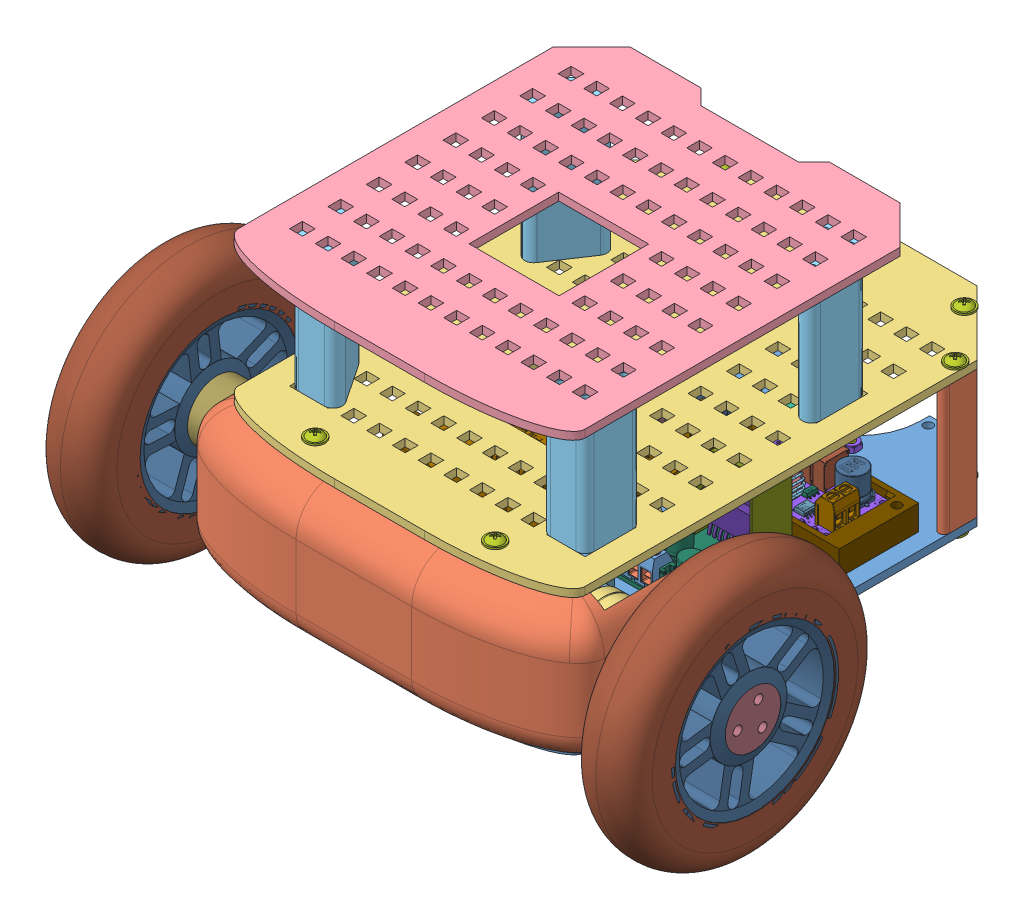
SolidWorks assembly main_assembly_generic, configuration Default. Lengths in mm.
Overall size (232.39 154.6 231.75).
188 component instances, 46 part files, 130 mates.
Components (placement in the parent):
- base_generic-1: base_generic [Predeterminado] at origin size (135.31 3.5 190.25)
- front_noah-1: front_noah [Predeterminado] at (0 3 75) size (155.37 50.11 66.16)
- JA25-371-12V-1: JA25-371-12V [Predeterminado] at (32.9354 21.1621 81.9623) x (0 0 -1) z (1 0 0) size (25 25 76.39)
  - Gearbox-1: Gearbox [Predeterminado] at (16.9623 5.2379 20.5646) size (25 25 21)
  - hub-1: hub [Predeterminado] at (16.9623 5.2379 39.5646) x (0.985611 -0.169031 0) z (0 0 1) size (6.95 6.95 4.5)
  - Motor-1: Motor [Predeterminado] at (16.9623 5.2379 -9.9354) size (24.2 24.2 30.5)
  - Axis-1: Axis [Predeterminado] at (16.9623 5.2379 39.5646) x (0.853161 0.521648 0) z (0 0 1) size (4 4 14)
  - PCB-1: PCB [Predeterminado] at (16.9623 5.2379 -11.4354) x (-1 0 0) z (0 0 -1) size (23 23 4.73)
  - Magnet-1: Magnet [Predeterminado] at (16.9623 5.2379 -17.3254) x (-0.17817 -0.984 0) z (0 0 -1) size (14.2 14.2 15.5)
- JA25-371-12V-2: JA25-371-12V [Predeterminado] at (-32.9354 21.1621 48.0377) x (0 0 1) z (-1 0 0) size (25 25 76.39)
  - Gearbox-1: Gearbox [Predeterminado] at (16.9623 5.2379 20.5646) size (25 25 21)
  - hub-1: hub [Predeterminado] at (16.9623 5.2379 39.5646) x (0.985611 -0.169031 0) z (0 0 1) size (6.95 6.95 4.5)
  - Motor-1: Motor [Predeterminado] at (16.9623 5.2379 -9.9354) size (24.2 24.2 30.5)
  - Axis-1: Axis [Predeterminado] at (16.9623 5.2379 39.5646) x (0.853161 0.521648 0) z (0 0 1) size (4 4 14)
  - PCB-1: PCB [Predeterminado] at (16.9623 5.2379 -11.4354) x (-1 0 0) z (0 0 -1) size (23 23 4.73)
  - Magnet-1: Magnet [Predeterminado] at (16.9623 5.2379 -17.3254) x (-0.17817 -0.984 0) z (0 0 -1) size (14.2 14.2 15.5)
- Arduino Uno-1: Arduino Uno [Default] at (-32.9854 13 -7.3988) x (0 0 -1) z (0 1 0) size (53 76.4 13)
- TuxsWheel100mm-1: TuxsWheel100mm [Default] at (-181.0669 -0.4628 121.5667) x (0 -0.425374 -0.905018) z (1 0 0) size (114.18 114.18 36.69)
  - B02-1: B02 [Default] at (39.7671 48.3733 64.9228) size (90.04 90.04 24)
  - B021-1: B021 [Default] at (39.7671 48.3733 64.9228) x (0.988174 0.153337 0) z (0 0 1) size (100.02 100.02 24.11)
  - Adapter1-1: Adapter1 [Default] at (39.7671 48.3733 72.3069) x (0 -1 0) z (0 0 1) size (23 23 29.26)
  - Adapter2-1: Adapter2 [Default] at (39.7671 48.3733 65.8069) x (0 -1 0) z (0 0 1) size (21.7 21.7 6.5)
  - countersunk flat head cross recess screw_din-6: countersunk flat head cross recess screw_din [DIN EN ISO 7046-1 - M3 x 10 - Z - 10C] at (51.0178 48.3733 97.0669) x (-1 0 0) z (0 -0.928088 -0.37236) size (10 5.5 5.5) (hidden)
  - countersunk flat head cross recess screw_din-7: countersunk flat head cross recess screw_din [DIN EN ISO 7046-1 - M3 x 10 - Z - 10C] at (28.4595 48.3733 97.0669) x (1 0 0) z (0 0.306192 0.95197) size (10 5.5 5.5) (hidden)
  - countersunk flat head cross recess screw_din-8: countersunk flat head cross recess screw_din [DIN EN ISO 7046-1 - M3 x 10 - Z - 10C] at (36.7671 53.5694 65.4069) x (0 0 1) z (-0.331366 0.943502 0) size (10 5.5 5.5) (hidden)
  - countersunk flat head cross recess screw_din-9: countersunk flat head cross recess screw_din [DIN EN ISO 7046-1 - M3 x 10 - Z - 10C] at (36.7671 43.1771 65.4069) x (0 0 1) z (-0.394756 0.918786 0) size (10 5.5 5.5) (hidden)
  - countersunk flat head cross recess screw_din-10: countersunk flat head cross recess screw_din [DIN EN ISO 7046-1 - M3 x 10 - Z - 10C] at (45.7671 48.3733 65.4069) x (0 0 1) z (0.637808 -0.770196 0) size (10 5.5 5.5) (hidden)
  - hex thin nut gradeb_din-1: hex thin nut gradeb_din [Hexagon Nut ISO 4036 - M3 - C] at (33.3451 48.3733 97.0669) x (0 -1 0) z (-1 0 0) size (5.5 6.35 1.8) (hidden)
  - hex thin nut gradeb_din-2: hex thin nut gradeb_din [Hexagon Nut ISO 4036 - M3 - C] at (44.1892 48.3733 97.0669) x (0 -1 0) z (-1 0 0) size (5.5 6.35 1.8) (hidden)
- TuxsWheel100mm-2: TuxsWheel100mm [Default] at (181.0669 87.718 52.2919) x (0 -0.778594 -0.627529) z (-1 0 0) size (114.18 114.18 36.69)
  - B02-1: B02 [Default] at (39.7671 48.3733 64.9228) size (90.04 90.04 24)
  - B021-1: B021 [Default] at (39.7671 48.3733 64.9228) x (0.988174 0.153337 0) z (0 0 1) size (100.02 100.02 24.11)
  - Adapter1-1: Adapter1 [Default] at (39.7671 48.3733 72.3069) x (0 -1 0) z (0 0 1) size (23 23 29.26)
  - Adapter2-1: Adapter2 [Default] at (39.7671 48.3733 65.8069) x (0 -1 0) z (0 0 1) size (21.7 21.7 6.5)
  - countersunk flat head cross recess screw_din-6: countersunk flat head cross recess screw_din [DIN EN ISO 7046-1 - M3 x 10 - Z - 10C] at (51.0178 48.3733 97.0669) x (-1 0 0) z (0 -0.928088 -0.37236) size (10 5.5 5.5) (hidden)
  - countersunk flat head cross recess screw_din-7: countersunk flat head cross recess screw_din [DIN EN ISO 7046-1 - M3 x 10 - Z - 10C] at (28.4595 48.3733 97.0669) x (1 0 0) z (0 0.306192 0.95197) size (10 5.5 5.5) (hidden)
  - countersunk flat head cross recess screw_din-8: countersunk flat head cross recess screw_din [DIN EN ISO 7046-1 - M3 x 10 - Z - 10C] at (36.7671 53.5694 65.4069) x (0 0 1) z (-0.331366 0.943502 0) size (10 5.5 5.5) (hidden)
  - countersunk flat head cross recess screw_din-9: countersunk flat head cross recess screw_din [DIN EN ISO 7046-1 - M3 x 10 - Z - 10C] at (36.7671 43.1771 65.4069) x (0 0 1) z (-0.394756 0.918786 0) size (10 5.5 5.5) (hidden)
  - countersunk flat head cross recess screw_din-10: countersunk flat head cross recess screw_din [DIN EN ISO 7046-1 - M3 x 10 - Z - 10C] at (45.7671 48.3733 65.4069) x (0 0 1) z (0.637808 -0.770196 0) size (10 5.5 5.5) (hidden)
  - hex thin nut gradeb_din-1: hex thin nut gradeb_din [Hexagon Nut ISO 4036 - M3 - C] at (33.3451 48.3733 97.0669) x (0 -1 0) z (-1 0 0) size (5.5 6.35 1.8) (hidden)
  - hex thin nut gradeb_din-2: hex thin nut gradeb_din [Hexagon Nut ISO 4036 - M3 - C] at (44.1892 48.3733 97.0669) x (0 -1 0) z (-1 0 0) size (5.5 6.35 1.8) (hidden)
- Spacer10mm-1: Spacer10mm [Varsayılan] at (-45 13 33) x (-0.837169 0 -0.546944) z (-0.546944 0 0.837169) size (5.71 16.2 5)
- Spacer10mm-2: Spacer10mm [Varsayılan] at (-45 13 -15.6) x (-0.837169 0 -0.546944) z (-0.546944 0 0.837169) size (5.71 16.2 5)
- Spacer10mm-3: Spacer10mm [Varsayılan] at (5.9048 13 -0.3747) x (-0.837169 0 -0.546944) z (-0.546944 0 0.837169) size (5.71 16.2 5)
- Spacer10mm-4: Spacer10mm [Varsayılan] at (5.9037 13 26.6253) x (-0.837169 0 -0.546944) z (-0.546944 0 0.837169) size (5.71 16.2 5)
- Montaj - L298 DC Motor Drive-1: Montaj - L298 DC Motor Drive [Varsayılan] at (35.2269 11.4274 -35.05) size (43.5 27 43.55)
  - L298 Board-1: L298 Board [Varsayılan] at (5.3531 1.5726 43.5) size (43.5 12.01 43.5)
  - Cooler Blok-1: Cooler Blok [Varsayılan] at (5.3531 27.5726 29.4518) x (-1 0 0) z (0 0 1) size (23 27 15.5)
  - L298N Regulator-1: L298N Regulator [Varsayılan] at (5.3531 16.3226 30.2018) size (21 23.01 4.5)
  - Vida M3x4.5-1: Vida M3x4.5 [Varsayılan] at (5.3531 22.0726 31.7018) size (5 5 6.5)
  - Clamp Body-1: Clamp Body [Varsayılan] at (-1.8969 8.5726 60.75) x (-1 0 0) z (0 0 -1) size (15 10.5 8)
  - Metal Clamp Part-1: Metal Clamp Part [Varsayılan] at (3.1031 6.5726 61.3938) size (4 11.02 6)
  - Metal Clamp Part-2: Metal Clamp Part [Varsayılan] at (-1.8969 6.5726 61.3938) size (4 11.02 6)
  - Metal Clamp Part-3: Metal Clamp Part [Varsayılan] at (-6.8969 6.5726 61.3938) size (4 11.02 6)
  - Clamp Body 2x-1: Clamp Body 2x [Varsayılan] at (-12.3969 8.5726 50.25) x (0 0 -1) z (1 0 0) size (10 10.5 8)
  - Metal Clamp Part-4: Metal Clamp Part [Varsayılan] at (-13.0407 6.5726 47.75) x (0 0 1) z (-1 0 0) size (4 11.02 6)
  - Metal Clamp Part-5: Metal Clamp Part [Varsayılan] at (-13.0407 6.5726 52.75) x (0 0 1) z (-1 0 0) size (4 11.02 6)
  - Clamp Body 2x-2: Clamp Body 2x [Varsayılan] at (23.1031 8.5726 50.25) x (0 0 1) z (-1 0 0) size (10 10.5 8)
  - Metal Clamp Part-6: Metal Clamp Part [Varsayılan] at (23.7469 6.5726 52.75) x (0 0 -1) z (1 0 0) size (4 11.02 6)
  - Metal Clamp Part-7: Metal Clamp Part [Varsayılan] at (23.7469 6.5726 47.75) x (0 0 -1) z (1 0 0) size (4 11.02 6)
- Spacer10mm-5: Spacer10mm [Varsayılan] at (20.83 13 28.2) x (-0.837169 0 -0.546944) z (-0.546944 0 0.837169) size (5.71 16.2 5)
- Spacer10mm-6: Spacer10mm [Varsayılan] at (20.83 13 -11.3) x (-0.837169 0 -0.546944) z (-0.546944 0 0.837169) size (5.71 16.2 5)
- Spacer10mm-7: Spacer10mm [Varsayılan] at (60.33 13 -11.3) x (-0.837169 0 -0.546944) z (-0.546944 0 0.837169) size (5.71 16.2 5)
- Spacer10mm-8: Spacer10mm [Varsayılan] at (60.33 13 28.2) x (-0.837169 0 -0.546944) z (-0.546944 0 0.837169) size (5.71 16.2 5)
- XL4015-1: XL4015 [Default] at (2.5 8.7 -25.3) x (1 0 0) z (0 1 0) size (51 26 18.44)
  - XL4015 StepDown DC-DC 5A (CC-CV) v1.step-1: XL4015 StepDown DC-DC 5A (CC-CV) v1.step [Default] at origin size (51 26 18.44)
    - Coil v9.step-1: Coil v9.step [Default] at (0 0 9) x (0 0 -1) z (0 -1 0) size (17.32 14.29 7.7)
      - Toro.step-1: Toro.step [Default] at (0.4 28 -5) size (13 12 6)
      - Spira.step-1: Spira.step [Default] at (0.4 28 -5) x (0.965926 0.258819 0) z (0 0 1) size (4.37 2.38 7.7)
      - Spira.step-2: Spira.step [Default] at (0.4 28 -5) x (0.866025 0.5 0) z (0 0 1) size (4.37 2.38 7.7)
      - Spira.step-3: Spira.step [Default] at (0.4 28 -5) x (0.707107 0.707107 0) z (0 0 1) size (4.37 2.38 7.7)
      - Spira.step-4: Spira.step [Default] at (0.4 28 -5) x (0.5 0.866025 0) z (0 0 1) size (4.37 2.38 7.7)
      - Spira.step-5: Spira.step [Default] at (0.4 28 -5) x (0.258819 0.965926 0) z (0 0 1) size (4.37 2.38 7.7)
      - Spira.step-6: Spira.step [Default] at (0.4 28 -5) x (0 1 0) z (0 0 1) size (4.37 2.38 7.7)
      - Spira.step-7: Spira.step [Default] at (0.4 28 -5) x (-0.258819 0.965926 0) z (0 0 1) size (4.37 2.38 7.7)
      - Spira.step-8: Spira.step [Default] at (0.4 28 -5) x (-0.5 0.866025 0) z (0 0 1) size (4.37 2.38 7.7)
      - Spira.step-9: Spira.step [Default] at (0.4 28 -5) x (-0.707107 0.707107 0) z (0 0 1) size (4.37 2.38 7.7)
      - Spira.step-10: Spira.step [Default] at (0.4 28 -5) x (-0.866025 0.5 0) z (0 0 1) size (4.37 2.38 7.7)
      - Spira.step-11: Spira.step [Default] at (0.4 28 -5) x (-0.965926 0.258819 0) z (0 0 1) size (4.37 2.38 7.7)
      - Spira.step-12: Spira.step [Default] at (0.4 28 -5) x (-1 0 0) z (0 0 1) size (4.37 2.38 7.7)
      - Spira.step-13: Spira.step [Default] at (0.4 28 -5) x (-0.965926 -0.258819 0) z (0 0 1) size (4.37 2.38 7.7)
      - Spira.step-14: Spira.step [Default] at (0.4 28 -5) x (-0.866025 -0.5 0) z (0 0 1) size (4.37 2.38 7.7)
      - Spira.step-15: Spira.step [Default] at (0.4 28 -5) x (-0.707107 -0.707107 0) z (0 0 1) size (4.37 2.38 7.7)
      - Spira.step-16: Spira.step [Default] at (0.4 28 -5) x (-0.5 -0.866025 0) z (0 0 1) size (4.37 2.38 7.7)
      - Spira.step-17: Spira.step [Default] at (0.4 28 -5) x (-0.258819 -0.965926 0) z (0 0 1) size (4.37 2.38 7.7)
      - Spira.step-18: Spira.step [Default] at (0.4 28 -5) x (0 -1 0) z (0 0 1) size (4.37 2.38 7.7)
      - Spira.step-19: Spira.step [Default] at (0.4 28 -5) x (0.258819 -0.965926 0) z (0 0 1) size (4.37 2.38 7.7)
      - Spira.step-20: Spira.step [Default] at (0.4 28 -5) x (0.5 -0.866025 0) z (0 0 1) size (4.37 2.38 7.7)
      - Spira.step-21: Spira.step [Default] at (0.4 28 -5) x (0.707107 -0.707107 0) z (0 0 1) size (4.37 2.38 7.7)
      - Spira.step-22: Spira.step [Default] at (0.4 28 -5) x (0.866025 -0.5 0) z (0 0 1) size (4.37 2.38 7.7)
      - SpiraCodA.step-1: SpiraCodA.step [Default] at (0.4015 27.9945 -5) x (1 0.000874 0) z (0 0 1) size (7.52 2.39 7.7)
      - SpiraCpdB.step-1: SpiraCpdB.step [Default] at (0.399 27.9963 -5) x (0.966079 -0.258245 0) z (0 0 1) size (7.28 3.27 7.7)
    - Basetta.step-1: Basetta.step [Default] at origin size (51 26 1.7)
    - DG301-5.0-02 v1.step-1: DG301-5.0-02 v1.step [Default] at (4 19.4 1.6) x (0 -1 0) z (0 0 1) size (10.6 7.6 14.3)
    - DG301-5.0-02 v1.step-2: DG301-5.0-02 v1.step [Default] at (47 6.6 1.6) x (0 1 0) z (0 0 1) size (10.6 7.6 14.3)
    - CAPACITOR 10x10 SMD v1.step-1: CAPACITOR 10x10 SMD v1.step [Default] at (9.325 5.925 1.6) x (1 0 0) z (0 -1 0) size (10.25 10.61 11.85)
    - CAPACITOR 10x10 SMD v1.step-2: CAPACITOR 10x10 SMD v1.step [Default] at (41.475 19.975 1.6) x (0 -1 0) z (-1 0 0) size (10.25 10.61 11.85)
    - Trimpot 3296W v1.step-1: Trimpot 3296W v1.step [Default] at (26.715 20.735 1.6) x (0 -1 0) z (0 0 1) size (9.56 4.83 14.15)
    - Trimpot 3296W v1.step-2: Trimpot 3296W v1.step [Default] at (32.265 20.735 1.6) x (0 -1 0) z (0 0 1) size (9.56 4.83 14.15)
    - DO-214AB v1.step-1: DO-214AB v1.step [Default] at (18.1 1.725 1.6) x (0 1 0) z (0 0 1) size (8.15 6.25 2.66)
    - XL4015 TO263-5-1 v1.step-1: XL4015 TO263-5-1 v1.step [Default] at (18.4666 17.0892 1.5654) x (0 -1 0) z (-0.006883 0 0.999976) size (9.82 14.6 4.22)
    - LM358 SOIC08 v1.step-1: LM358 SOIC08 v1.step [Default] at (37 6 1.55) x (0 -1 0) z (0 0 1) size (5 6.17 2.02)
    - UPC78L08T-E1-AZ.step-1: UPC78L08T-E1-AZ.step [Default] at (31.81 12.82 1.6) x (0 1 0) z (0 0 1) size (4.36 4 1.51)
    - SC-59A v1.step-1: SC-59A v1.step [Default] at (36.8 13.75 1.6) x (0 -1 0) z (0 0 1) size (3.1 3 1.45)
    - LED v1.step-1: LED v1.step [Default] at (44.84 1.625 1.62) x (0 -1 0) z (-1 0 0) size (1.27 0.67 2.02)
    - LED v1.step-2: LED v1.step [Default] at (39.84 1.625 1.62) x (0 -1 0) z (-1 0 0) size (1.27 0.67 2.02)
    - LED v1.step-3: LED v1.step [Default] at (20.16 23.875 1.62) x (0 -1 0) z (-1 0 0) size (1.27 0.67 2.02)
- XL4015-2: XL4015 [Default] at (-2.5 8.7 -51.3) x (-1 0 0) z (0 1 0) size (51 26 18.44)
  - XL4015 StepDown DC-DC 5A (CC-CV) v1.step-1: XL4015 StepDown DC-DC 5A (CC-CV) v1.step [Default] at origin size (51 26 18.44)
    - Coil v9.step-1: Coil v9.step [Default] at (0 0 9) x (0 0 -1) z (0 -1 0) size (17.32 14.29 7.7)
      - Toro.step-1: Toro.step [Default] at (0.4 28 -5) size (13 12 6)
      - Spira.step-1: Spira.step [Default] at (0.4 28 -5) x (0.965926 0.258819 0) z (0 0 1) size (4.37 2.38 7.7)
      - Spira.step-2: Spira.step [Default] at (0.4 28 -5) x (0.866025 0.5 0) z (0 0 1) size (4.37 2.38 7.7)
      - Spira.step-3: Spira.step [Default] at (0.4 28 -5) x (0.707107 0.707107 0) z (0 0 1) size (4.37 2.38 7.7)
      - Spira.step-4: Spira.step [Default] at (0.4 28 -5) x (0.5 0.866025 0) z (0 0 1) size (4.37 2.38 7.7)
      - Spira.step-5: Spira.step [Default] at (0.4 28 -5) x (0.258819 0.965926 0) z (0 0 1) size (4.37 2.38 7.7)
      - Spira.step-6: Spira.step [Default] at (0.4 28 -5) x (0 1 0) z (0 0 1) size (4.37 2.38 7.7)
      - Spira.step-7: Spira.step [Default] at (0.4 28 -5) x (-0.258819 0.965926 0) z (0 0 1) size (4.37 2.38 7.7)
      - Spira.step-8: Spira.step [Default] at (0.4 28 -5) x (-0.5 0.866025 0) z (0 0 1) size (4.37 2.38 7.7)
      - Spira.step-9: Spira.step [Default] at (0.4 28 -5) x (-0.707107 0.707107 0) z (0 0 1) size (4.37 2.38 7.7)
      - Spira.step-10: Spira.step [Default] at (0.4 28 -5) x (-0.866025 0.5 0) z (0 0 1) size (4.37 2.38 7.7)
      - Spira.step-11: Spira.step [Default] at (0.4 28 -5) x (-0.965926 0.258819 0) z (0 0 1) size (4.37 2.38 7.7)
      - Spira.step-12: Spira.step [Default] at (0.4 28 -5) x (-1 0 0) z (0 0 1) size (4.37 2.38 7.7)
      - Spira.step-13: Spira.step [Default] at (0.4 28 -5) x (-0.965926 -0.258819 0) z (0 0 1) size (4.37 2.38 7.7)
      - Spira.step-14: Spira.step [Default] at (0.4 28 -5) x (-0.866025 -0.5 0) z (0 0 1) size (4.37 2.38 7.7)
      - Spira.step-15: Spira.step [Default] at (0.4 28 -5) x (-0.707107 -0.707107 0) z (0 0 1) size (4.37 2.38 7.7)
      - Spira.step-16: Spira.step [Default] at (0.4 28 -5) x (-0.5 -0.866025 0) z (0 0 1) size (4.37 2.38 7.7)
      - Spira.step-17: Spira.step [Default] at (0.4 28 -5) x (-0.258819 -0.965926 0) z (0 0 1) size (4.37 2.38 7.7)
      - Spira.step-18: Spira.step [Default] at (0.4 28 -5) x (0 -1 0) z (0 0 1) size (4.37 2.38 7.7)
      - Spira.step-19: Spira.step [Default] at (0.4 28 -5) x (0.258819 -0.965926 0) z (0 0 1) size (4.37 2.38 7.7)
      - Spira.step-20: Spira.step [Default] at (0.4 28 -5) x (0.5 -0.866025 0) z (0 0 1) size (4.37 2.38 7.7)
      - Spira.step-21: Spira.step [Default] at (0.4 28 -5) x (0.707107 -0.707107 0) z (0 0 1) size (4.37 2.38 7.7)
      - Spira.step-22: Spira.step [Default] at (0.4 28 -5) x (0.866025 -0.5 0) z (0 0 1) size (4.37 2.38 7.7)
      - SpiraCodA.step-1: SpiraCodA.step [Default] at (0.4015 27.9945 -5) x (1 0.000874 0) z (0 0 1) size (7.52 2.39 7.7)
      - SpiraCpdB.step-1: SpiraCpdB.step [Default] at (0.399 27.9963 -5) x (0.966079 -0.258245 0) z (0 0 1) size (7.28 3.27 7.7)
    - Basetta.step-1: Basetta.step [Default] at origin size (51 26 1.7)
    - DG301-5.0-02 v1.step-1: DG301-5.0-02 v1.step [Default] at (4 19.4 1.6) x (0 -1 0) z (0 0 1) size (10.6 7.6 14.3)
    - DG301-5.0-02 v1.step-2: DG301-5.0-02 v1.step [Default] at (47 6.6 1.6) x (0 1 0) z (0 0 1) size (10.6 7.6 14.3)
    - CAPACITOR 10x10 SMD v1.step-1: CAPACITOR 10x10 SMD v1.step [Default] at (9.325 5.925 1.6) x (1 0 0) z (0 -1 0) size (10.25 10.61 11.85)
    - CAPACITOR 10x10 SMD v1.step-2: CAPACITOR 10x10 SMD v1.step [Default] at (41.475 19.975 1.6) x (0 -1 0) z (-1 0 0) size (10.25 10.61 11.85)
    - Trimpot 3296W v1.step-1: Trimpot 3296W v1.step [Default] at (26.715 20.735 1.6) x (0 -1 0) z (0 0 1) size (9.56 4.83 14.15)
    - Trimpot 3296W v1.step-2: Trimpot 3296W v1.step [Default] at (32.265 20.735 1.6) x (0 -1 0) z (0 0 1) size (9.56 4.83 14.15)
    - DO-214AB v1.step-1: DO-214AB v1.step [Default] at (18.1 1.725 1.6) x (0 1 0) z (0 0 1) size (8.15 6.25 2.66)
    - XL4015 TO263-5-1 v1.step-1: XL4015 TO263-5-1 v1.step [Default] at (18.4666 17.0892 1.5654) x (0 -1 0) z (-0.006883 0 0.999976) size (9.82 14.6 4.22)
    - LM358 SOIC08 v1.step-1: LM358 SOIC08 v1.step [Default] at (37 6 1.55) x (0 -1 0) z (0 0 1) size (5 6.17 2.02)
    - UPC78L08T-E1-AZ.step-1: UPC78L08T-E1-AZ.step [Default] at (31.81 12.82 1.6) x (0 1 0) z (0 0 1) size (4.36 4 1.51)
    - SC-59A v1.step-1: SC-59A v1.step [Default] at (36.8 13.75 1.6) x (0 -1 0) z (0 0 1) size (3.1 3 1.45)
    - LED v1.step-1: LED v1.step [Default] at (44.84 1.625 1.62) x (0 -1 0) z (-1 0 0) size (1.27 0.67 2.02)
    - LED v1.step-2: LED v1.step [Default] at (39.84 1.625 1.62) x (0 -1 0) z (-1 0 0) size (1.27 0.67 2.02)
    - LED v1.step-3: LED v1.step [Default] at (20.16 23.875 1.62) x (0 -1 0) z (-1 0 0) size (1.27 0.67 2.02)
- SMPS_support-2: SMPS_support [Default] at (0 3 -38.3) size (122 9.7 31)
- back_left-1: back_left [Default] at (-65.5 3 -69.1716) x (0.707107 0 0.707107) z (-0.707107 0 0.707107) size (11.07 50 43.07)
- back_right-1: back_right [Default] at (65.5 3 -69.1716) x (0.707107 0 -0.707107) z (0.707107 0 0.707107) size (11.07 50 43.07)
- top_generic-1: top_generic [Predeterminado] at (0 53 0) size (135.31 3.5 190.25)
- shelf_generic-1: shelf_generic [Default] at (0 106 20) size (135.31 3.5 150.25)
- Spacer50mm-1: Spacer50mm [Default] at (46.264 106 -17.4479) x (-1 0 0) z (0 0 1) size (17 50 22)
- Spacer50mm-2: Spacer50mm [Default] at (46.264 56 52.4479) x (-1 0 0) z (0 0 -1) size (17 50 22)
- Spacer50mm-3: Spacer50mm [Default] at (-46.264 56 -17.4479) size (17 50 22)
- Spacer50mm-4: Spacer50mm [Default] at (-46.264 106 52.4479) x (1 0 0) z (0 0 -1) size (17 50 22)
- caster_generic-3: caster_generic [Default] at (0 0 -69.0197) x (-1 0 0) z (0 0 1) size (50 21 32)
- pan head cross collar screw_din-1: pan head cross collar screw_din [DIN 967 - M3 x 10 - Z --- 9N] at (27.5 -2.35 50) x (0 1 0) z (0 0 1) size (12.25 7.5 7.5)
- pan head cross collar screw_din-2: pan head cross collar screw_din [DIN 967 - M3 x 10 - Z --- 9N] at (50 -2.35 85) x (0 1 0) z (0 0 1) size (12.25 7.5 7.5)
- pan head cross collar screw_din-3: pan head cross collar screw_din [DIN 967 - M3 x 10 - Z --- 9N] at (19.5 -3.85 -69.0197) x (0 1 0) z (-0.624185 0 0.781276) size (12.25 7.5 7.5)
- pan head cross collar screw_din-4: pan head cross collar screw_din [DIN 967 - M3 x 10 - Z --- 9N] at (-19.5 -3.85 -69.0197) x (0 1 0) z (0.6712 0 -0.741276) size (12.25 7.5 7.5)
- pan head cross collar screw_din-5: pan head cross collar screw_din [DIN 967 - M3 x 10 - Z --- 9N] at (-27.5 -2.35 50) x (0 1 0) z (0 0 1) size (12.25 7.5 7.5)
- pan head cross collar screw_din-6: pan head cross collar screw_din [DIN 967 - M3 x 10 - Z --- 9N] at (-50 -2.35 85) x (0 1 0) z (0 0 1) size (12.25 7.5 7.5)
- hex nut style 1 gradeab_din-1: hex nut style 1 gradeab_din [Hexagon Nut ISO 4032 - M3 - W - N] at (-19.5 3 -69.0197) x (1 0 0) z (0 -1 0) size (5.5 6.35 2.4)
- hex nut style 1 gradeab_din-2: hex nut style 1 gradeab_din [Hexagon Nut ISO 4032 - M3 - W - N] at (19.5 3 -69.0197) x (1 0 0) z (0 -1 0) size (5.5 6.35 2.4)
- pan head cross collar screw_din-7: pan head cross collar screw_din [DIN 967 - M3 x 10 - Z --- 9N] at (57.5 -2.35 -50.8) x (0 1 0) z (-0.624185 0 0.781276) size (12.25 7.5 7.5)
- pan head cross collar screw_din-8: pan head cross collar screw_din [DIN 967 - M3 x 10 - Z --- 9N] at (-57.5 -2.35 -27.8) x (0 1 0) z (-0.624185 0 0.781276) size (12.25 7.5 7.5)
- hex thin nut gradeb_din-1: hex thin nut gradeb_din [Hexagon Nut ISO 4036 - M3 - N] at (5.9 -1.8 -0.37) x (1 0 0) z (0 -1 0) size (5.5 6.35 1.8)
- hex thin nut gradeb_din-2: hex thin nut gradeb_din [Hexagon Nut ISO 4036 - M3 - N] at (20.83 -1.8 28.2) x (1 0 0) z (0 -1 0) size (5.5 6.35 1.8)
- hex thin nut gradeb_din-3: hex thin nut gradeb_din [Hexagon Nut ISO 4036 - M3 - N] at (-45 -1.8 -15.6) x (1 0 0) z (0 -1 0) size (5.5 6.35 1.8)
- hex thin nut gradeb_din-4: hex thin nut gradeb_din [Hexagon Nut ISO 4036 - M3 - N] at (-45 -1.8 33) x (1 0 0) z (0 -1 0) size (5.5 6.35 1.8)
- hex thin nut gradeb_din-5: hex thin nut gradeb_din [Hexagon Nut ISO 4036 - M3 - N] at (20.83 -1.8 -11.3) x (1 0 0) z (0 -1 0) size (5.5 6.35 1.8)
- hex thin nut gradeb_din-6: hex thin nut gradeb_din [Hexagon Nut ISO 4036 - M3 - N] at (60.33 -1.8 28.2) x (1 0 0) z (0 -1 0) size (5.5 6.35 1.8)
- hex thin nut gradeb_din-7: hex thin nut gradeb_din [Hexagon Nut ISO 4036 - M3 - N] at (60.33 -1.8 -11.3) x (1 0 0) z (0 -1 0) size (5.5 6.35 1.8)
- hex thin nut gradeb_din-8: hex thin nut gradeb_din [Hexagon Nut ISO 4036 - M3 - N] at (5.9 -1.8 26.63) x (1 0 0) z (0 -1 0) size (5.5 6.35 1.8)
- pan head cross collar screw_din-9: pan head cross collar screw_din [DIN 967 - M3 x 10 - Z --- 9N] at (-64 -2.35 -65) x (0 1 0) z (-0.624185 0 0.781276) size (12.25 7.5 7.5)
- pan head cross collar screw_din-10: pan head cross collar screw_din [DIN 967 - M3 x 10 - Z --- 9N] at (-47.3475 -2.35 -85.2028) x (0 1 0) z (-0.624185 0 0.781276) size (12.25 7.5 7.5)
- pan head cross collar screw_din-11: pan head cross collar screw_din [DIN 967 - M3 x 10 - Z --- 9N] at (64 -2.35 -65) x (0 1 0) z (-0.624185 0 0.781276) size (12.25 7.5 7.5)
- pan head cross collar screw_din-12: pan head cross collar screw_din [DIN 967 - M3 x 10 - Z --- 9N] at (47.3475 -2.35 -85.2028) x (0 1 0) z (-0.624185 0 0.781276) size (12.25 7.5 7.5)
- pan head cross collar screw_din-13: pan head cross collar screw_din [DIN 967 - M3 x 10 - Z --- 9N] at (-64 58.35 -65) x (0 -1 0) z (0.666726 0 0.745303) size (12.25 7.5 7.5)
- pan head cross collar screw_din-14: pan head cross collar screw_din [DIN 967 - M3 x 10 - Z --- 9N] at (64 58.35 -65) x (0 -1 0) z (0.666726 0 0.745303) size (12.25 7.5 7.5)
- pan head cross collar screw_din-15: pan head cross collar screw_din [DIN 967 - M3 x 10 - Z --- 9N] at (-35 58.35 85) x (0 -1 0) z (0.666726 0 0.745303) size (12.25 7.5 7.5)
- pan head cross collar screw_din-16: pan head cross collar screw_din [DIN 967 - M3 x 10 - Z --- 9N] at (35 58.35 85) x (0 -1 0) z (0.666726 0 0.745303) size (12.25 7.5 7.5)
- pan head cross collar screw_din-17: pan head cross collar screw_din [DIN 967 - M3 x 10 - Z --- 9N] at (47.3475 58.35 -85.2028) x (0 -1 0) z (0.666726 0 0.745303) size (12.25 7.5 7.5)
- pan head cross collar screw_din-18: pan head cross collar screw_din [DIN 967 - M3 x 10 - Z --- 9N] at (-47.3475 58.35 -85.2028) x (0 -1 0) z (0.666726 0 0.745303) size (12.25 7.5 7.5)
Mates (geometry in assembly coordinates):
- Coincident1: coincident anti-aligned: plane of base_generic-1 through (0 3 0) normal (0 1 0); plane of front_noah-1 through (0 3 75) normal (0 -1 0)
- Concentric1: concentric anti-aligned: cylinder of base_generic-1 through (-50 0 85) axis (0 1 0) radius 1.75; cylinder of front_noah-1 through (-50 13 85) axis (0 -1 0) radius 1.5
- Concentric2: concentric anti-aligned: cylinder of base_generic-1 through (27.5 0 50) axis (0 1 0) radius 1.75; cylinder of front_noah-1 through (27.5 13 50) axis (0 -1 0) radius 1.5
- Concentric3: concentric aligned: cylinder of front_noah-1 through (77.775 26.4 65) axis (-1 0 0) radius 3.75; cylinder of JA25-371-12V-1/hub-1 through (77 26.4 65) axis (-1 0 0) radius 3.475
- Concentric4: concentric anti-aligned: cylinder of front_noah-1 through (77.775 26.4 73.75) axis (-1 0 0) radius 1.75; cylinder of JA25-371-12V-1/Gearbox-1 through (53.5 26.4 73.75) axis (1 0 0) radius 1.5
- Coincident2: coincident anti-aligned: plane of front_noah-1 through (74.5 26.4 65) normal (-1 0 0); plane of JA25-371-12V-1/Gearbox-1 through (74.5 26.4 65) normal (1 0 0)
- Coincident3: coincident anti-aligned: plane of front_noah-1 through (-74.5 -146.1643 45) normal (1 0 0); plane of JA25-371-12V-2/Gearbox-1 through (-74.5 26.4 65) normal (-1 0 0)
- Concentric5: concentric anti-aligned: cylinder of front_noah-1 through (77.775 26.4 65) axis (-1 0 0) radius 3.75; cylinder of JA25-371-12V-2/hub-1 through (-77 26.4 65) axis (1 0 0) radius 3.475
- Concentric6: concentric aligned: cylinder of front_noah-1 through (77.775 26.4 56.25) axis (-1 0 0) radius 1.75; cylinder of JA25-371-12V-2/Gearbox-1 through (-53.5 26.4 56.25) axis (-1 0 0) radius 1.5
- Concentric7: concentric anti-aligned: cylinder of JA25-371-12V-1/Axis-1 through (86.5 26.4 65) axis (-1 0 0) radius 2; cylinder of TuxsWheel100mm-2/Adapter1-1 through (99.5 26.4 65) axis (1 0 0) radius 2.1
- Distance1: distance = 2 mm anti-aligned: plane of TuxsWheel100mm-2/Adapter1-1 through (79.5 26.4 65) normal (-1 0 0); plane of front_noah-1 through (77.5 53 45) normal (1 0 0)
- Concentric8: concentric anti-aligned: cylinder of JA25-371-12V-2/Axis-1 through (-86.5 26.4 65) axis (1 0 0) radius 2; cylinder of TuxsWheel100mm-1/Adapter1-1 through (-99.5 26.4 65) axis (-1 0 0) radius 2.1
- Distance2: distance = 2 mm anti-aligned: plane of front_noah-1 through (-77.5 53 45) normal (-1 0 0); plane of TuxsWheel100mm-1/Adapter1-1 through (-79.5 26.4 65) normal (1 0 0)
- Coincident4: coincident anti-aligned: plane of base_generic-1 through (0 3 0) normal (0 1 0); plane of Spacer10mm-1 through (-45 3 33) normal (0 -1 0)
- Coincident5: coincident anti-aligned: plane of base_generic-1 through (0 3 0) normal (0 1 0); plane of Spacer10mm-2 through (-45 3 -15.6) normal (0 -1 0)
- Coincident6: coincident anti-aligned: plane of base_generic-1 through (0 3 0) normal (0 1 0); plane of Spacer10mm-3 through (5.9048 3 -0.3747) normal (0 -1 0)
- Coincident7: coincident anti-aligned: plane of base_generic-1 through (0 3 0) normal (0 1 0); plane of Spacer10mm-4 through (5.9037 3 26.6253) normal (0 -1 0)
- Concentric9: concentric aligned: cylinder of Arduino Uno-1 through (-45 7 -15.6) axis (0 1 0) radius 2; cylinder of Spacer10mm-2 through (-45 7 -15.6) axis (0 1 0) radius 1.365
- Coincident8: coincident anti-aligned: plane of Arduino Uno-1 through (-32.9854 13 -7.3988) normal (0 -1 0); plane of Spacer10mm-2 through (-45 13 -15.6) normal (0 1 0)
- Concentric10: concentric aligned: cylinder of Arduino Uno-1 through (5.9048 7 -0.3747) axis (0 1 0) radius 2; cylinder of Spacer10mm-3 through (5.9048 7 -0.3747) axis (0 1 0) radius 1.365
- Coincident9: coincident anti-aligned: plane of Arduino Uno-1 through (-32.9854 13 -7.3988) normal (0 -1 0); plane of Spacer10mm-3 through (5.9048 13 -0.3747) normal (0 1 0)
- Concentric11: concentric aligned: cylinder of Arduino Uno-1 through (-45 7 33) axis (0 1 0) radius 2; cylinder of Spacer10mm-1 through (-45 7 33) axis (0 1 0) radius 1.365
- Concentric12: concentric aligned: cylinder of Arduino Uno-1 through (5.9037 7 26.6253) axis (0 1 0) radius 2; cylinder of Spacer10mm-4 through (5.9037 7 26.6253) axis (0 1 0) radius 1.365
- Coincident10: coincident anti-aligned: plane of Arduino Uno-1 through (-32.9854 13 -7.3988) normal (0 -1 0); plane of Spacer10mm-4 through (5.9037 13 26.6253) normal (0 1 0)
- Concentric13: concentric anti-aligned: cylinder of base_generic-1 through (-45 3.25 33) axis (0 -1 0) radius 1.75; cylinder of Spacer10mm-1 through (-45 1.8 33) axis (0 1 0) radius 1.3375
- Parallel1: parallel aligned: plane of base_generic-1 through (-67.5 3 -95) normal (-1 0 0); plane of Arduino Uno-1 through (-59.3365 15 35.2) normal (-1 0 0)
- Coincident12: coincident anti-aligned: plane of base_generic-1 through (0 3 0) normal (0 1 0); plane of Spacer10mm-5 through (20.83 3 28.2) normal (0 -1 0)
- Coincident13: coincident anti-aligned: plane of base_generic-1 through (0 3 0) normal (0 1 0); plane of Spacer10mm-8 through (60.33 3 28.2) normal (0 -1 0)
- Coincident14: coincident anti-aligned: plane of base_generic-1 through (0 3 0) normal (0 1 0); plane of Spacer10mm-7 through (60.33 3 -11.3) normal (0 -1 0)
- Coincident15: coincident anti-aligned: plane of base_generic-1 through (0 3 0) normal (0 1 0); plane of Spacer10mm-6 through (20.83 3 -11.3) normal (0 -1 0)
- Coincident16: coincident anti-aligned: plane of Montaj - L298 DC Motor Drive-1/L298 Board-1 through (40.58 13 8.45) normal (0 -1 0); plane of Spacer10mm-7 through (60.33 13 -11.3) normal (0 1 0)
- Concentric14: concentric anti-aligned: cylinder of Montaj - L298 DC Motor Drive-1/L298 Board-1 through (60.33 14.5 -11.3) axis (0 -1 0) radius 1.5; cylinder of Spacer10mm-7 through (60.33 7 -11.3) axis (0 1 0) radius 1.365
- Concentric15: concentric anti-aligned: cylinder of Montaj - L298 DC Motor Drive-1/L298 Board-1 through (60.33 14.5 28.2) axis (0 -1 0) radius 1.5; cylinder of Spacer10mm-8 through (60.33 7 28.2) axis (0 1 0) radius 1.365
- Concentric16: concentric anti-aligned: cylinder of Montaj - L298 DC Motor Drive-1/L298 Board-1 through (20.83 14.5 28.2) axis (0 -1 0) radius 1.5; cylinder of Spacer10mm-5 through (20.83 7 28.2) axis (0 1 0) radius 1.365
- Concentric17: concentric anti-aligned: cylinder of Montaj - L298 DC Motor Drive-1/L298 Board-1 through (20.83 14.5 -11.3) axis (0 -1 0) radius 1.5; cylinder of Spacer10mm-6 through (20.83 7 -11.3) axis (0 1 0) radius 1.365
- Concentric18: concentric anti-aligned: cylinder of base_generic-1 through (20.83 -0.25 28.2) axis (0 1 0) radius 1.75; cylinder of Montaj - L298 DC Motor Drive-1/L298 Board-1 through (20.83 14.5 28.2) axis (0 -1 0) radius 1.5
- Concentric19: concentric anti-aligned: cylinder of base_generic-1 through (60.33 -0.25 -11.3) axis (0 1 0) radius 1.75; cylinder of Montaj - L298 DC Motor Drive-1/L298 Board-1 through (60.33 14.5 -11.3) axis (0 -1 0) radius 1.5
- Coincident28: coincident anti-aligned: plane of base_generic-1 through (0 3 0) normal (0 1 0); plane of SMPS_support-2 through (0 3 -38.3) normal (0 -1 0)
- Distance7: distance = 0.5 mm anti-aligned: plane of XL4015-1/XL4015 StepDown DC-DC 5A (CC-CV) v1.step-1/Basetta.step-1 through (53.5 8.7 -51.3) normal (0 0 -1); plane of SMPS_support-2 through (54 -55.5918 -51.8) normal (0 0 1)
- Distance8: distance = 0.5 mm anti-aligned: plane of XL4015-1/XL4015 StepDown DC-DC 5A (CC-CV) v1.step-1/Basetta.step-1 through (53.5 8.7 -25.3) normal (1 0 0); plane of SMPS_support-2 through (54 -55.5918 -51.8) normal (-1 0 0)
- Coincident33: coincident anti-aligned: plane of XL4015-1/XL4015 StepDown DC-DC 5A (CC-CV) v1.step-1/DG301-5.0-02 v1.step-2 through (49.5 6 -36.9) normal (0 -1 0); plane of SMPS_support-2 through (0 6 -38.3) normal (0 1 0)
- Coincident34: coincident anti-aligned: plane of XL4015-2/XL4015 StepDown DC-DC 5A (CC-CV) v1.step-1/DG301-5.0-02 v1.step-1 through (-6.5 6 -31.9) normal (0 -1 0); plane of SMPS_support-2 through (0 6 -38.3) normal (0 1 0)
- Distance12: distance = 0.5 mm anti-aligned: plane of SMPS_support-2 through (-54 -55.5918 -24.8) normal (0 0 -1); plane of XL4015-2/XL4015 StepDown DC-DC 5A (CC-CV) v1.step-1/Basetta.step-1 through (-53.5 8.7 -25.3) normal (0 0 1)
- Distance13: distance = 0.5 mm anti-aligned: plane of SMPS_support-2 through (-2 -55.5918 -51.8) normal (-1 0 0); plane of XL4015-2/XL4015 StepDown DC-DC 5A (CC-CV) v1.step-1/Basetta.step-1 through (-2.5 8.7 -25.3) normal (1 0 0)
- Distance14: distance = 6.5 mm aligned: plane of base_generic-1 through (67.5 3 -95) normal (1 0 0); plane of SMPS_support-2 through (61 12.7 -53.8) normal (1 0 0)
- Distance15: distance = 5 mm anti-aligned: plane of Arduino Uno-1 through (-59.3365 15 -17.8) normal (0 0 -1); plane of SMPS_support-2 through (-61 12.7 -22.8) normal (0 0 1)
- Coincident42: coincident aligned: plane of base_generic-1 through (-67.5 3 -70) normal (-0.707107 0 -0.707107); plane of back-1 through (-44.2868 53 -93.2132) normal (-0.707107 0 -0.707107)
- Coincident43: coincident anti-aligned: plane of base_generic-1 through (0 3 0) normal (0 1 0); plane of back-1 through (-42.8726 3 -91.799) normal (0 -1 0)
- Coincident44: coincident aligned: plane of base_generic-1 through (-67.5 3 -95) normal (-1 0 0); plane of back-1 through (-67.5 53 -70) normal (-1 0 0)
- Coincident45: coincident anti-aligned: plane of base_generic-1 through (0 3 0) normal (0 1 0); plane of back_right-1 through (42.8726 3 -91.799) normal (0 -1 0)
- Concentric20: concentric anti-aligned: cylinder of base_generic-1 through (47.3475 -0.25 -85.2028) axis (0 1 0) radius 1.75; cylinder of back_right-1 through (47.3475 53 -85.2028) axis (0 -1 0) radius 1.5
- Concentric23: concentric anti-aligned: cylinder of base_generic-1 through (64 -0.25 -65) axis (0 1 0) radius 1.75; cylinder of back_right-1 through (64 53 -65) axis (0 -1 0) radius 1.5
- Coincident46: coincident anti-aligned: plane of front_noah-1 through (0 53 75) normal (0 1 0); plane of top_generic-1 through (0 53 0) normal (0 -1 0)
- Concentric24: concentric aligned: cylinder of front_noah-1 through (35 43 85) axis (0 1 0) radius 1.5; cylinder of top_generic-1 through (35 46 85) axis (0 1 0) radius 1.75
- Concentric25: concentric aligned: cylinder of front_noah-1 through (-35 43 85) axis (0 1 0) radius 1.5; cylinder of top_generic-1 through (-35 46 85) axis (0 1 0) radius 1.75
- Coincident47: coincident anti-aligned: plane of top_generic-1 through (0 56 0) normal (0 1 0); plane of Spacer50mm-3 through (-54 56 -34) normal (0 -1 0)
- Coincident52: coincident anti-aligned: plane of top_generic-1 through (0 56 0) normal (0 1 0); plane of Spacer50mm-4 through (-54 56 69) normal (0 -1 0)
- Coincident54: coincident anti-aligned: plane of top_generic-1 through (0 56 0) normal (0 1 0); plane of Spacer50mm-1 through (54 56 -34) normal (0 -1 0)
- Coincident55: coincident aligned: plane of Spacer50mm-1 through (54 56 -37.5) normal (0 0 -1); plane of Spacer50mm-3 through (-54 106 -37.5) normal (0 0 -1)
- Coincident59: coincident anti-aligned: plane of top_generic-1 through (0 56 0) normal (0 1 0); plane of Spacer50mm-2 through (54 56 69) normal (0 -1 0)
- Coincident60: coincident aligned: plane of Spacer50mm-1 through (57.5 56 -34) normal (1 0 0); plane of Spacer50mm-2 through (57.5 106 69) normal (1 0 0)
- Coincident61: coincident aligned: plane of Spacer50mm-3 through (-57.5 106 -34) normal (-1 0 0); plane of Spacer50mm-4 through (-57.5 56 69) normal (-1 0 0)
- Parallel3: parallel aligned: plane of top_generic-1 through (-67.5 56 -95) normal (-1 0 0); plane of Spacer50mm-4 through (-57.5 56 69) normal (-1 0 0)
- Coincident63: coincident anti-aligned: line of top_generic-1 through (-57.5 56 72.5) axis (1 0 0); line of Spacer50mm-4 through (-44 56 72.5) axis (-1 0 0)
- Coincident64: coincident: line of top_generic-1 through (-57.5 56 67.5) axis (0 0 1); plane of Spacer50mm-4 through (-57.5 56 69) normal (-1 0 0)
- Coincident65: coincident aligned: line of top_generic-1 through (57.5 56 72.5) axis (0 0 -1); line of Spacer50mm-2 through (57.5 56 69) axis (0 0 -1)
- Coincident66: coincident aligned: line of Spacer50mm-2 through (44 56 72.5) axis (1 0 0); line of top_generic-1 through (52.5 56 72.5) axis (1 0 0)
- Coincident68: coincident anti-aligned: plane of shelf_noah-1 through (0 106 20) normal (0 -1 0); plane of Spacer50mm-4 through (-54 106 69) normal (0 1 0)
- Coincident69: coincident aligned: plane of top_generic-1 through (-67.5 56 95) normal (0 0 1); plane of shelf_noah-1 through (-67.5 109 95) normal (0 0 1)
- Coincident70: coincident aligned: plane of top_generic-1 through (67.5 56 -95) normal (1 0 0); plane of shelf_noah-1 through (67.5 109 -55) normal (1 0 0)
- Coincident72: coincident: line of top_generic-1 through (47.5 56 -37.5) axis (-1 0 0); plane of Spacer50mm-1 through (54 56 -37.5) normal (0 0 -1)
- Coincident75: coincident anti-aligned: plane of base_generic-1 through (0 0 0) normal (0 -1 0); plane of caster_generic-3 through (0 0 -69.0197) normal (0 1 0)
- Concentric31: concentric anti-aligned: cylinder of base_generic-1 through (19.5 10 -69.0197) axis (0 -1 0) radius 1.75; cylinder of caster_generic-3 through (19.5 -1.5 -69.0197) axis (0 1 0) radius 1.75
- Concentric34: concentric anti-aligned: cylinder of base_generic-1 through (-19.5 10 -69.0197) axis (0 -1 0) radius 1.75; cylinder of caster_generic-3 through (-19.5 -1.5 -69.0197) axis (0 1 0) radius 1.75
- Coincident78: coincident anti-aligned: plane of base_generic-1 through (0 0 0) normal (0 -1 0); plane of pan head cross collar screw_din-1 through (26 0 50) normal (0 1 0)
- Coincident79: coincident anti-aligned: plane of base_generic-1 through (0 0 0) normal (0 -1 0); plane of pan head cross collar screw_din-2 through (48.5 0 85) normal (0 1 0)
- Coincident80: coincident anti-aligned: plane of base_generic-1 through (0 0 0) normal (0 -1 0); plane of pan head cross collar screw_din-5 through (-29 0 50) normal (0 1 0)
- Coincident81: coincident anti-aligned: plane of base_generic-1 through (0 0 0) normal (0 -1 0); plane of pan head cross collar screw_din-6 through (-51.5 0 85) normal (0 1 0)
- Concentric36: concentric anti-aligned: circle of base_generic-1; cylinder of pan head cross collar screw_din-1 through (27.5 -8.7 50) axis (0 -1 0) radius 1.5
- Concentric37: concentric anti-aligned: cylinder of base_generic-1 through (50 0 85) axis (0 1 0) radius 1.75; cylinder of pan head cross collar screw_din-2 through (50 -8.7 85) axis (0 -1 0) radius 1.5
- Concentric38: concentric anti-aligned: circle of base_generic-1; cylinder of pan head cross collar screw_din-6 through (-50 -8.7 85) axis (0 -1 0) radius 1.5
- Concentric39: concentric anti-aligned: cylinder of base_generic-1 through (-27.5 0 50) axis (0 1 0) radius 1.75; cylinder of pan head cross collar screw_din-5 through (-27.5 -8.7 50) axis (0 -1 0) radius 1.5
- Concentric40: concentric aligned: cylinder of base_generic-1 through (19.5 10 -69.0197) axis (0 -1 0) radius 1.75; cylinder of pan head cross collar screw_din-3 through (19.5 -10.2 -69.0197) axis (0 -1 0) radius 1.5
- Concentric41: concentric aligned: cylinder of base_generic-1 through (-19.5 10 -69.0197) axis (0 -1 0) radius 1.75; cylinder of pan head cross collar screw_din-4 through (-19.5 -10.2 -69.0197) axis (0 -1 0) radius 1.5
- Coincident82: coincident anti-aligned: plane of caster_generic-3 through (0 -1.5 -69.0197) normal (0 -1 0); plane of pan head cross collar screw_din-4 through (-18.3881 -1.5 -68.0129) normal (0 1 0)
- Coincident83: coincident anti-aligned: plane of caster_generic-3 through (0 -1.5 -69.0197) normal (0 -1 0); plane of pan head cross collar screw_din-3 through (18.3281 -1.5 -69.9559) normal (0 1 0)
- Coincident84: coincident anti-aligned: plane of base_generic-1 through (0 3 0) normal (0 1 0); plane of hex nut style 1 gradeab_din-1 through (-19.5 3 -65.8442) normal (0 -1 0)
- Coincident85: coincident anti-aligned: plane of base_generic-1 through (0 3 0) normal (0 1 0); plane of hex nut style 1 gradeab_din-2 through (19.5 3 -65.8442) normal (0 -1 0)
- Concentric42: concentric aligned: cylinder of pan head cross collar screw_din-4 through (-19.5 -10.2 -69.0197) axis (0 -1 0) radius 1.5; cylinder of hex nut style 1 gradeab_din-1 through (-19.5 5.4 -69.0197) axis (0 -1 0) radius 1.25
- Concentric43: concentric aligned: cylinder of pan head cross collar screw_din-3 through (19.5 -10.2 -69.0197) axis (0 -1 0) radius 1.5; cylinder of hex nut style 1 gradeab_din-2 through (19.5 5.4 -69.0197) axis (0 -1 0) radius 1.25
- Concentric44: concentric anti-aligned: cylinder of base_generic-1 through (57.5 -0.25 -50.8) axis (0 1 0) radius 1.75; cylinder of pan head cross collar screw_din-7 through (57.5 -8.7 -50.8) axis (0 -1 0) radius 1.5
- Coincident86: coincident anti-aligned: plane of base_generic-1 through (0 0 0) normal (0 -1 0); plane of pan head cross collar screw_din-7 through (56.3281 0 -51.7363) normal (0 1 0)
- Concentric46: concentric anti-aligned: cylinder of base_generic-1 through (-57.5 -0.25 -27.8) axis (0 1 0) radius 1.75; cylinder of pan head cross collar screw_din-8 through (-57.5 -8.7 -27.8) axis (0 -1 0) radius 1.5
- Coincident88: coincident anti-aligned: plane of base_generic-1 through (0 0 0) normal (0 -1 0); plane of pan head cross collar screw_din-8 through (-58.6719 0 -28.7363) normal (0 1 0)
- Coincident89: coincident anti-aligned: plane of base_generic-1 through (0 0 0) normal (0 -1 0); plane of hex thin nut gradeb_din-3 through (-45 0 -12.4246) normal (0 1 0)
- Coincident90: coincident anti-aligned: plane of base_generic-1 through (0 0 0) normal (0 -1 0); plane of hex thin nut gradeb_din-2 through (20.83 0 31.3754) normal (0 1 0)
- Coincident91: coincident anti-aligned: plane of base_generic-1 through (0 0 0) normal (0 -1 0); plane of hex thin nut gradeb_din-1 through (5.9 0 2.8054) normal (0 1 0)
- Coincident92: coincident anti-aligned: plane of base_generic-1 through (0 0 0) normal (0 -1 0); plane of hex thin nut gradeb_din-4 through (-45 0 36.1754) normal (0 1 0)
- Coincident93: coincident anti-aligned: plane of base_generic-1 through (0 0 0) normal (0 -1 0); plane of hex thin nut gradeb_din-5 through (20.83 0 -8.1246) normal (0 1 0)
- Coincident94: coincident anti-aligned: plane of base_generic-1 through (0 0 0) normal (0 -1 0); plane of hex thin nut gradeb_din-6 through (60.33 0 31.3754) normal (0 1 0)
- Coincident95: coincident anti-aligned: plane of base_generic-1 through (0 0 0) normal (0 -1 0); plane of hex thin nut gradeb_din-8 through (5.9 0 29.8054) normal (0 1 0)
- Coincident96: coincident anti-aligned: plane of base_generic-1 through (0 0 0) normal (0 -1 0); plane of hex thin nut gradeb_din-7 through (60.33 0 -8.1246) normal (0 1 0)
- Concentric47: concentric anti-aligned: cylinder of Spacer10mm-2 through (-45 1.8 -15.6) axis (0 1 0) radius 1.3375; cylinder of hex thin nut gradeb_din-3 through (-45 0 -15.6) axis (0 -1 0) radius 1.25
- Concentric48: concentric anti-aligned: cylinder of base_generic-1 through (20.83 -0.25 -11.3) axis (0 1 0) radius 1.75; cylinder of hex thin nut gradeb_din-5 through (20.83 0 -11.3) axis (0 -1 0) radius 1.25
- Concentric49: concentric anti-aligned: cylinder of base_generic-1 through (60.33 -0.25 -11.3) axis (0 1 0) radius 1.75; cylinder of hex thin nut gradeb_din-7 through (60.33 0 -11.3) axis (0 -1 0) radius 1.25
- Concentric50: concentric aligned: cylinder of base_generic-1 through (5.9 3.25 -0.37) axis (0 -1 0) radius 1.75; cylinder of hex thin nut gradeb_din-1 through (5.9 0 -0.37) axis (0 -1 0) radius 1.25
- Concentric51: concentric anti-aligned: cylinder of base_generic-1 through (60.33 -0.25 28.2) axis (0 1 0) radius 1.75; cylinder of hex thin nut gradeb_din-6 through (60.33 0 28.2) axis (0 -1 0) radius 1.25
- Concentric52: concentric anti-aligned: cylinder of base_generic-1 through (20.83 -0.25 28.2) axis (0 1 0) radius 1.75; cylinder of hex thin nut gradeb_din-2 through (20.83 0 28.2) axis (0 -1 0) radius 1.25
- Concentric53: concentric aligned: cylinder of base_generic-1 through (5.9 3.25 26.63) axis (0 -1 0) radius 1.75; cylinder of hex thin nut gradeb_din-8 through (5.9 0 26.63) axis (0 -1 0) radius 1.25
- Concentric54: concentric aligned: cylinder of base_generic-1 through (-45 3.25 33) axis (0 -1 0) radius 1.75; cylinder of hex thin nut gradeb_din-4 through (-45 0 33) axis (0 -1 0) radius 1.25
- Coincident97: coincident anti-aligned: plane of base_generic-1 through (0 0 0) normal (0 -1 0); plane of pan head cross collar screw_din-10 through (-48.5194 0 -86.1391) normal (0 1 0)
- Coincident98: coincident anti-aligned: plane of base_generic-1 through (0 0 0) normal (0 -1 0); plane of pan head cross collar screw_din-9 through (-65.1719 0 -65.9363) normal (0 1 0)
- Coincident99: coincident anti-aligned: plane of base_generic-1 through (0 0 0) normal (0 -1 0); plane of pan head cross collar screw_din-12 through (46.1755 0 -86.1391) normal (0 1 0)
- Coincident100: coincident aligned: plane of base_generic-1 through (0 0 0) normal (0 -1 0); circle of pan head cross collar screw_din-11
- Concentric55: concentric anti-aligned: cylinder of base_generic-1 through (64 -0.25 -65) axis (0 1 0) radius 1.75; cylinder of pan head cross collar screw_din-11 through (64 -8.7 -65) axis (0 -1 0) radius 1.5
- Concentric56: concentric anti-aligned: circle of base_generic-1; cylinder of pan head cross collar screw_din-12 through (47.3475 -8.7 -85.2028) axis (0 -1 0) radius 1.5
- Concentric57: concentric anti-aligned: cylinder of base_generic-1 through (-47.3475 -0.25 -85.2028) axis (0 1 0) radius 1.75; cylinder of pan head cross collar screw_din-10 through (-47.3475 -8.7 -85.2028) axis (0 -1 0) radius 1.5
- Concentric58: concentric anti-aligned: cylinder of base_generic-1 through (-64 -0.25 -65) axis (0 1 0) radius 1.75; cylinder of pan head cross collar screw_din-9 through (-64 -8.7 -65) axis (0 -1 0) radius 1.5
- Concentric59: concentric aligned: cylinder of top_generic-1 through (-64 46 -65) axis (0 1 0) radius 1.5; cylinder of pan head cross collar screw_din-13 through (-64 64.7 -65) axis (0 1 0) radius 1.5
- Coincident101: coincident anti-aligned: plane of top_generic-1 through (0 56 0) normal (0 1 0); plane of pan head cross collar screw_din-13 through (-62.882 56 -66.0001) normal (0 -1 0)
- Concentric60: concentric aligned: cylinder of top_generic-1 through (-47.3475 46 -85.2028) axis (0 1 0) radius 1.5; cylinder of pan head cross collar screw_din-18 through (-47.3475 64.7 -85.2028) axis (0 1 0) radius 1.5
- Concentric61: concentric aligned: cylinder of top_generic-1 through (47.3475 46 -85.2028) axis (0 1 0) radius 1.5; cylinder of pan head cross collar screw_din-17 through (47.3475 64.7 -85.2028) axis (0 1 0) radius 1.5
- Concentric62: concentric aligned: cylinder of top_generic-1 through (64 46 -65) axis (0 1 0) radius 1.5; cylinder of pan head cross collar screw_din-14 through (64 64.7 -65) axis (0 1 0) radius 1.5
- Concentric63: concentric aligned: cylinder of top_generic-1 through (35 46 85) axis (0 1 0) radius 1.75; cylinder of pan head cross collar screw_din-16 through (35 64.7 85) axis (0 1 0) radius 1.5
- Concentric64: concentric aligned: cylinder of top_generic-1 through (-35 46 85) axis (0 1 0) radius 1.75; cylinder of pan head cross collar screw_din-15 through (-35 64.7 85) axis (0 1 0) radius 1.5
- Coincident102: coincident anti-aligned: plane of top_generic-1 through (0 56 0) normal (0 1 0); plane of pan head cross collar screw_din-16 through (36.118 56 83.9999) normal (0 -1 0)
- Coincident103: coincident anti-aligned: plane of top_generic-1 through (0 56 0) normal (0 1 0); plane of pan head cross collar screw_din-15 through (-33.882 56 83.9999) normal (0 -1 0)
- Coincident104: coincident anti-aligned: plane of top_generic-1 through (0 56 0) normal (0 1 0); plane of pan head cross collar screw_din-18 through (-46.2295 56 -86.2029) normal (0 -1 0)
- Coincident105: coincident anti-aligned: plane of top_generic-1 through (0 56 0) normal (0 1 0); plane of pan head cross collar screw_din-17 through (48.4654 56 -86.2029) normal (0 -1 0)
- Coincident106: coincident anti-aligned: plane of top_generic-1 through (0 56 0) normal (0 1 0); plane of pan head cross collar screw_din-14 through (65.118 56 -66.0001) normal (0 -1 0)
